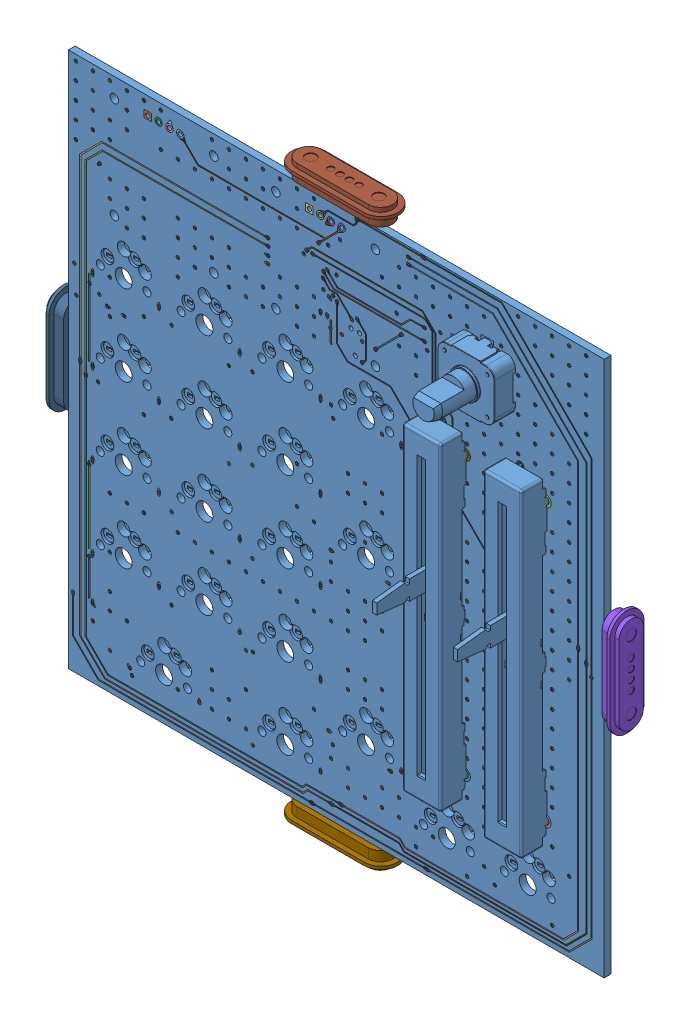
SolidWorks assembly Modulu1, configuration Default. Lengths in mm. (continued)
Components (placement in the parent): (continued)
- Numpad test 2.step-1: Numpad test 2.step [Default] at origin size (134.6 135 22.98) (continued)
  - Numpad test 21175.step-1: Numpad test 21175.step [Default] at origin size (0.81 0.81 0.01)
  - Numpad test 21176.step-1: Numpad test 21176.step [Default] at origin size (0.81 0.81 0.01)
  - Numpad test 21177.step-1: Numpad test 21177.step [Default] at origin size (0.81 0.81 0.01)
  - Numpad test 21178.step-1: Numpad test 21178.step [Default] at origin size (0.81 0.81 0.01)
  - Numpad test 21179.step-1: Numpad test 21179.step [Default] at origin size (0.81 0.81 0.01)
  - Numpad test 21180.step-1: Numpad test 21180.step [Default] at origin size (0.81 0.81 0.01)
  - Numpad test 21181.step-1: Numpad test 21181.step [Default] at origin size (0.81 0.81 0.01)
  - Numpad test 21182.step-1: Numpad test 21182.step [Default] at origin size (0.81 0.81 0.01)
  - Numpad test 21183.step-1: Numpad test 21183.step [Default] at origin size (0.81 0.81 0.01)
  - Numpad test 21184.step-1: Numpad test 21184.step [Default] at origin size (0.81 0.81 0.01)
  - Numpad test 21185.step-1: Numpad test 21185.step [Default] at origin size (0.81 0.81 0.01)
  - Numpad test 21186.step-1: Numpad test 21186.step [Default] at origin size (0.81 0.81 0.01)
  - Numpad test 21187.step-1: Numpad test 21187.step [Default] at origin size (0.81 0.81 0.01)
  - Numpad test 21188.step-1: Numpad test 21188.step [Default] at origin size (0.81 0.81 0.01)
  - Numpad test 21189.step-1: Numpad test 21189.step [Default] at origin size (0.81 0.81 0.01)
  - Numpad test 21190.step-1: Numpad test 21190.step [Default] at origin size (0.81 0.81 0.01)
  - Numpad test 21191.step-1: Numpad test 21191.step [Default] at origin size (0.81 0.81 0.01)
  - Numpad test 21192.step-1: Numpad test 21192.step [Default] at origin size (0.81 0.81 0.01)
  - Numpad test 21193.step-1: Numpad test 21193.step [Default] at origin size (0.81 0.81 0.01)
  - Numpad test 21194.step-1: Numpad test 21194.step [Default] at origin size (0.81 0.81 0.01)
  - Numpad test 21195.step-1: Numpad test 21195.step [Default] at origin size (0.81 0.81 0.01)
  - Numpad test 21196.step-1: Numpad test 21196.step [Default] at origin size (0.81 0.81 0.01)
  - Numpad test 21197.step-1: Numpad test 21197.step [Default] at origin size (0.81 0.81 0.01)
  - Numpad test 21198.step-1: Numpad test 21198.step [Default] at origin size (0.81 0.81 0.01)
  - Numpad test 21199.step-1: Numpad test 21199.step [Default] at origin size (0.81 0.81 0.01)
  - Numpad test 21200.step-1: Numpad test 21200.step [Default] at origin size (0.81 0.81 0.01)
  - Numpad test 21201.step-1: Numpad test 21201.step [Default] at origin size (0.81 0.81 0.01)
  - Numpad test 21202.step-1: Numpad test 21202.step [Default] at origin size (0.81 0.81 0.01)
  - Numpad test 21203.step-1: Numpad test 21203.step [Default] at origin size (0.81 0.81 0.01)
  - Numpad test 21204.step-1: Numpad test 21204.step [Default] at origin size (0.81 0.81 0.01)
  - Numpad test 21205.step-1: Numpad test 21205.step [Default] at origin size (0.81 0.81 0.01)
  - Numpad test 21206.step-1: Numpad test 21206.step [Default] at origin size (0.81 0.81 0.01)
  - Numpad test 21207.step-1: Numpad test 21207.step [Default] at origin size (0.81 0.81 0.01)
  - Numpad test 21208.step-1: Numpad test 21208.step [Default] at origin size (0.81 0.81 0.01)
  - Numpad test 21209.step-1: Numpad test 21209.step [Default] at origin size (0.81 0.81 0.01)
  - Numpad test 21210.step-1: Numpad test 21210.step [Default] at origin size (0.81 0.81 0.01)
  - Numpad test 21211.step-1: Numpad test 21211.step [Default] at origin size (0.81 0.81 0.01)
  - Numpad test 21212.step-1: Numpad test 21212.step [Default] at origin size (0.81 0.81 0.01)
  - Numpad test 21213.step-1: Numpad test 21213.step [Default] at origin size (0.81 0.81 0.01)
  - Numpad test 21214.step-1: Numpad test 21214.step [Default] at origin size (0.81 0.81 0.01)
  - Numpad test 21215.step-1: Numpad test 21215.step [Default] at origin size (0.81 0.81 0.01)
  - Numpad test 21216.step-1: Numpad test 21216.step [Default] at origin size (0.81 0.81 0.01)
  - Numpad test 21217.step-1: Numpad test 21217.step [Default] at origin size (0.81 0.81 0.01)
  - Numpad test 21218.step-1: Numpad test 21218.step [Default] at origin size (0.81 0.81 0.01)
  - Numpad test 21219.step-1: Numpad test 21219.step [Default] at origin size (0.81 0.81 0.01)
  - Numpad test 21220.step-1: Numpad test 21220.step [Default] at origin size (0.81 0.81 0.01)
  - Numpad test 21221.step-1: Numpad test 21221.step [Default] at origin size (0.81 0.81 0.01)
  - Numpad test 21222.step-1: Numpad test 21222.step [Default] at origin size (0.81 0.81 0.01)
  - Numpad test 21223.step-1: Numpad test 21223.step [Default] at origin size (0.81 0.81 0.01)
  - Numpad test 21224.step-1: Numpad test 21224.step [Default] at origin size (0.81 0.81 0.01)
  - Numpad test 21225.step-1: Numpad test 21225.step [Default] at origin size (0.81 0.81 0.01)
  - Numpad test 21226.step-1: Numpad test 21226.step [Default] at origin size (0.81 0.81 0.01)
  - Numpad test 21227.step-1: Numpad test 21227.step [Default] at origin size (0.81 0.81 0.01)
  - Numpad test 21228.step-1: Numpad test 21228.step [Default] at origin size (0.81 0.81 0.01)
  - Numpad test 21229.step-1: Numpad test 21229.step [Default] at origin size (0.81 0.81 0.01)
  - Numpad test 21230.step-1: Numpad test 21230.step [Default] at origin size (0.81 0.81 0.01)
  - Numpad test 21231.step-1: Numpad test 21231.step [Default] at origin size (0.81 0.81 0.01)
  - Numpad test 21232.step-1: Numpad test 21232.step [Default] at origin size (0.81 0.81 0.01)
  - Numpad test 21233.step-1: Numpad test 21233.step [Default] at origin size (0.81 0.81 0.01)
  - Numpad test 21234.step-1: Numpad test 21234.step [Default] at origin size (0.81 0.81 0.01)
  - Numpad test 21235.step-1: Numpad test 21235.step [Default] at origin size (0.81 0.81 0.01)
  - Numpad test 21236.step-1: Numpad test 21236.step [Default] at origin size (0.81 0.81 0.01)
  - Numpad test 21237.step-1: Numpad test 21237.step [Default] at origin size (0.81 0.81 0.01)
  - Numpad test 21238.step-1: Numpad test 21238.step [Default] at origin size (0.81 0.81 0.01)
  - Numpad test 21239.step-1: Numpad test 21239.step [Default] at origin size (0.81 0.81 0.01)
  - Numpad test 21240.step-1: Numpad test 21240.step [Default] at origin size (0.81 0.81 0.01)
  - Numpad test 21241.step-1: Numpad test 21241.step [Default] at origin size (0.81 0.81 0.01)
  - Numpad test 21242.step-1: Numpad test 21242.step [Default] at origin size (0.81 0.81 0.01)
  - Numpad test 21243.step-1: Numpad test 21243.step [Default] at origin size (0.81 0.81 0.01)
  - Numpad test 21244.step-1: Numpad test 21244.step [Default] at origin size (0.81 0.81 0.01)
  - Numpad test 21245.step-1: Numpad test 21245.step [Default] at origin size (0.81 0.81 0.01)
  - Numpad test 21246.step-1: Numpad test 21246.step [Default] at origin size (0.81 0.81 0.01)
  - Numpad test 21247.step-1: Numpad test 21247.step [Default] at origin size (0.81 0.81 0.01)
  - Numpad test 21248.step-1: Numpad test 21248.step [Default] at origin size (0.81 0.81 0.01)
  - Numpad test 21249.step-1: Numpad test 21249.step [Default] at origin size (0.81 0.81 0.01)
  - Numpad test 21250.step-1: Numpad test 21250.step [Default] at origin size (0.81 0.81 0.01)
  - Numpad test 21251.step-1: Numpad test 21251.step [Default] at origin size (0.81 0.81 0.01)
  - Numpad test 21252.step-1: Numpad test 21252.step [Default] at origin size (0.81 0.81 0.01)
  - Numpad test 21253.step-1: Numpad test 21253.step [Default] at origin size (0.81 0.81 0.01)
  - Numpad test 21254.step-1: Numpad test 21254.step [Default] at origin size (0.81 0.81 0.01)
  - Numpad test 21255.step-1: Numpad test 21255.step [Default] at origin size (0.81 0.81 0.01)
  - Numpad test 21256.step-1: Numpad test 21256.step [Default] at origin size (0.81 0.81 0.01)
  - Numpad test 21257.step-1: Numpad test 21257.step [Default] at origin size (0.81 0.81 0.01)
  - Numpad test 21258.step-1: Numpad test 21258.step [Default] at origin size (0.81 0.81 0.01)
  - Numpad test 21259.step-1: Numpad test 21259.step [Default] at origin size (0.81 0.81 0.01)
  - Numpad test 21260.step-1: Numpad test 21260.step [Default] at origin size (0.81 0.81 0.01)
  - Numpad test 21261.step-1: Numpad test 21261.step [Default] at origin size (0.81 0.81 0.01)
  - Numpad test 21262.step-1: Numpad test 21262.step [Default] at origin size (0.81 0.81 0.01)
  - Numpad test 21263.step-1: Numpad test 21263.step [Default] at origin size (0.81 0.81 0.01)
  - Numpad test 21264.step-1: Numpad test 21264.step [Default] at origin size (0.81 0.81 0.01)
  - Numpad test 21265.step-1: Numpad test 21265.step [Default] at origin size (0.81 0.81 0.01)
  - Numpad test 21266.step-1: Numpad test 21266.step [Default] at origin size (0.81 0.81 0.01)
  - Numpad test 21267.step-1: Numpad test 21267.step [Default] at origin size (0.81 0.81 0.01)
  - Numpad test 21268.step-1: Numpad test 21268.step [Default] at origin size (0.81 0.81 0.01)
  - Numpad test 21269.step-1: Numpad test 21269.step [Default] at origin size (0.81 0.81 0.01)
  - Numpad test 21270.step-1: Numpad test 21270.step [Default] at origin size (0.81 0.81 0.01)
  - Numpad test 21271.step-1: Numpad test 21271.step [Default] at origin size (0.81 0.81 0.01)
  - Numpad test 21272.step-1: Numpad test 21272.step [Default] at origin size (0.81 0.81 0.01)
  - Numpad test 21273.step-1: Numpad test 21273.step [Default] at origin size (0.81 0.81 0.01)
  - Numpad test 21274.step-1: Numpad test 21274.step [Default] at origin size (0.81 0.81 0.01)
  - Numpad test 21275.step-1: Numpad test 21275.step [Default] at origin size (0.81 0.81 0.01)
  - Numpad test 21276.step-1: Numpad test 21276.step [Default] at origin size (0.81 0.81 0.01)
  - Numpad test 21277.step-1: Numpad test 21277.step [Default] at origin size (0.81 0.81 0.01)
  - Numpad test 21278.step-1: Numpad test 21278.step [Default] at origin size (0.81 0.81 0.01)
  - Numpad test 21279.step-1: Numpad test 21279.step [Default] at origin size (0.81 0.81 0.01)
  - Numpad test 21280.step-1: Numpad test 21280.step [Default] at origin size (0.81 0.81 0.01)
  - Numpad test 21281.step-1: Numpad test 21281.step [Default] at origin size (0.81 0.81 0.01)
  - Numpad test 21282.step-1: Numpad test 21282.step [Default] at origin size (0.81 0.81 0.01)
  - Numpad test 21283.step-1: Numpad test 21283.step [Default] at origin size (0.81 0.81 0.01)
  - Numpad test 21284.step-1: Numpad test 21284.step [Default] at origin size (0.81 0.81 0.01)
  - Numpad test 21285.step-1: Numpad test 21285.step [Default] at origin size (0.81 0.81 0.01)
  - Numpad test 21286.step-1: Numpad test 21286.step [Default] at origin size (0.81 0.81 0.01)
  - Numpad test 21287.step-1: Numpad test 21287.step [Default] at origin size (0.81 0.81 0.01)
  - Numpad test 21288.step-1: Numpad test 21288.step [Default] at origin size (0.81 0.81 0.01)
  - Numpad test 21289.step-1: Numpad test 21289.step [Default] at origin size (0.81 0.81 0.01)
  - Numpad test 21290.step-1: Numpad test 21290.step [Default] at origin size (0.81 0.81 0.01)
  - Numpad test 21291.step-1: Numpad test 21291.step [Default] at origin size (0.81 0.81 0.01)
  - Numpad test 21292.step-1: Numpad test 21292.step [Default] at origin size (0.81 0.81 0.01)
  - Numpad test 21293.step-1: Numpad test 21293.step [Default] at origin size (0.81 0.81 0.01)
  - Numpad test 21294.step-1: Numpad test 21294.step [Default] at origin size (0.81 0.81 0.01)
  - Numpad test 21295.step-1: Numpad test 21295.step [Default] at origin size (0.81 0.81 0.01)
  - Numpad test 21296.step-1: Numpad test 21296.step [Default] at origin size (0.81 0.81 0.01)
  - Numpad test 21297.step-1: Numpad test 21297.step [Default] at origin size (0.81 0.81 0.01)
  - Numpad test 21298.step-1: Numpad test 21298.step [Default] at origin size (0.81 0.81 0.01)
  - Numpad test 21299.step-1: Numpad test 21299.step [Default] at origin size (0.81 0.81 0.01)
  - Numpad test 21300.step-1: Numpad test 21300.step [Default] at origin size (0.81 0.81 0.01)
  - Numpad test 21301.step-1: Numpad test 21301.step [Default] at origin size (0.81 0.81 0.01)
  - Numpad test 21302.step-1: Numpad test 21302.step [Default] at origin size (0.81 0.81 0.01)
  - Numpad test 21303.step-1: Numpad test 21303.step [Default] at origin size (0.81 0.81 0.01)
  - Numpad test 21304.step-1: Numpad test 21304.step [Default] at origin size (0.81 0.81 0.01)
  - Numpad test 21305.step-1: Numpad test 21305.step [Default] at origin size (0.81 0.81 0.01)
  - Numpad test 21306.step-1: Numpad test 21306.step [Default] at origin size (0.81 0.81 0.01)
  - Numpad test 21307.step-1: Numpad test 21307.step [Default] at origin size (0.81 0.81 0.01)
  - Numpad test 21308.step-1: Numpad test 21308.step [Default] at origin size (0.81 0.81 0.01)
  - Numpad test 21309.step-1: Numpad test 21309.step [Default] at origin size (0.81 0.81 0.01)
  - Numpad test 21310.step-1: Numpad test 21310.step [Default] at origin size (0.81 0.81 0.01)
  - Numpad test 21311.step-1: Numpad test 21311.step [Default] at origin size (0.81 0.81 0.01)
  - Numpad test 21312.step-1: Numpad test 21312.step [Default] at origin size (0.81 0.81 0.01)
  - Numpad test 21313.step-1: Numpad test 21313.step [Default] at origin size (0.81 0.81 0.01)
  - Numpad test 21314.step-1: Numpad test 21314.step [Default] at origin size (0.81 0.81 0.01)
  - Numpad test 21315.step-1: Numpad test 21315.step [Default] at origin size (0.81 0.81 0.01)
  - Numpad test 21316.step-1: Numpad test 21316.step [Default] at origin size (0.81 0.81 0.01)
  - Numpad test 21317.step-1: Numpad test 21317.step [Default] at origin size (0.81 0.81 0.01)
  - Numpad test 21318.step-1: Numpad test 21318.step [Default] at origin size (0.81 0.81 0.01)
  - Numpad test 21319.step-1: Numpad test 21319.step [Default] at origin size (0.81 0.81 0.01)
  - Numpad test 21320.step-1: Numpad test 21320.step [Default] at origin size (0.81 0.81 0.01)
  - Numpad test 21321.step-1: Numpad test 21321.step [Default] at origin size (0.81 0.81 0.01)
  - Numpad test 21322.step-1: Numpad test 21322.step [Default] at origin size (0.81 0.81 0.01)
  - Numpad test 21323.step-1: Numpad test 21323.step [Default] at origin size (0.81 0.81 0.01)
  - Numpad test 21324.step-1: Numpad test 21324.step [Default] at origin size (0.81 0.81 0.01)
  - Numpad test 21325.step-1: Numpad test 21325.step [Default] at origin size (0.81 0.81 0.01)
  - Numpad test 21326.step-1: Numpad test 21326.step [Default] at origin size (0.81 0.81 0.01)
  - Numpad test 21327.step-1: Numpad test 21327.step [Default] at origin size (0.81 0.81 0.01)
  - Numpad test 21328.step-1: Numpad test 21328.step [Default] at origin size (0.81 0.81 0.01)
  - Numpad test 21329.step-1: Numpad test 21329.step [Default] at origin size (0.81 0.81 0.01)
  - Numpad test 21330.step-1: Numpad test 21330.step [Default] at origin size (0.81 0.81 0.01)
  - Numpad test 21331.step-1: Numpad test 21331.step [Default] at origin size (0.81 0.81 0.01)
  - Numpad test 21332.step-1: Numpad test 21332.step [Default] at origin size (0.81 0.81 0.01)
  - Numpad test 21333.step-1: Numpad test 21333.step [Default] at origin size (0.81 0.81 0.01)
  - Numpad test 21334.step-1: Numpad test 21334.step [Default] at origin size (0.81 0.81 0.01)
  - Numpad test 21335.step-1: Numpad test 21335.step [Default] at origin size (0.81 0.81 0.01)
  - Numpad test 21336.step-1: Numpad test 21336.step [Default] at origin size (0.81 0.81 0.01)
  - Numpad test 21337.step-1: Numpad test 21337.step [Default] at origin size (0.81 0.81 0.01)
  - Numpad test 21338.step-1: Numpad test 21338.step [Default] at origin size (0.81 0.81 0.01)
  - Numpad test 21339.step-1: Numpad test 21339.step [Default] at origin size (0.81 0.81 0.01)
  - Numpad test 21340.step-1: Numpad test 21340.step [Default] at origin size (0.81 0.81 0.01)
  - Numpad test 21341.step-1: Numpad test 21341.step [Default] at origin size (0.81 0.81 0.01)
  - Numpad test 21342.step-1: Numpad test 21342.step [Default] at origin size (0.81 0.81 0.01)
  - Numpad test 21343.step-1: Numpad test 21343.step [Default] at origin size (0.81 0.81 0.01)
  - Numpad test 21344.step-1: Numpad test 21344.step [Default] at origin size (0.81 0.81 0.01)
  - Numpad test 21345.step-1: Numpad test 21345.step [Default] at origin size (0.81 0.81 0.01)
  - Numpad test 21346.step-1: Numpad test 21346.step [Default] at origin size (0.81 0.81 0.01)
  - Numpad test 21347.step-1: Numpad test 21347.step [Default] at origin size (0.81 0.81 0.01)
  - Numpad test 21348.step-1: Numpad test 21348.step [Default] at origin size (0.81 0.81 0.01)
  - Numpad test 21349.step-1: Numpad test 21349.step [Default] at origin size (0.81 0.81 0.01)
  - Numpad test 21350.step-1: Numpad test 21350.step [Default] at origin size (0.81 0.81 0.01)
  - Numpad test 21351.step-1: Numpad test 21351.step [Default] at origin size (0.81 0.81 0.01)
  - Numpad test 21352.step-1: Numpad test 21352.step [Default] at origin size (0.81 0.81 0.01)
  - Numpad test 21353.step-1: Numpad test 21353.step [Default] at origin size (0.81 0.81 0.01)
  - Numpad test 21354.step-1: Numpad test 21354.step [Default] at origin size (0.81 0.81 0.01)
  - Numpad test 21355.step-1: Numpad test 21355.step [Default] at origin size (0.81 0.81 0.01)
  - Numpad test 21356.step-1: Numpad test 21356.step [Default] at origin size (0.81 0.81 0.01)
  - Numpad test 21357.step-1: Numpad test 21357.step [Default] at origin size (0.81 0.81 0.01)
  - Numpad test 21358.step-1: Numpad test 21358.step [Default] at origin size (0.81 0.81 0.01)
  - Numpad test 21359.step-1: Numpad test 21359.step [Default] at origin size (0.81 0.81 0.01)
  - Numpad test 21360.step-1: Numpad test 21360.step [Default] at origin size (0.81 0.81 0.01)
  - Numpad test 21361.step-1: Numpad test 21361.step [Default] at origin size (0.81 0.81 0.01)
  - Numpad test 21362.step-1: Numpad test 21362.step [Default] at origin size (0.81 0.81 0.01)
  - Numpad test 21363.step-1: Numpad test 21363.step [Default] at origin size (0.81 0.81 0.01)
  - Numpad test 21364.step-1: Numpad test 21364.step [Default] at origin size (0.81 0.81 0.01)
  - Numpad test 21365.step-1: Numpad test 21365.step [Default] at origin size (0.81 0.81 0.01)
  - Numpad test 21366.step-1: Numpad test 21366.step [Default] at origin size (0.81 0.81 0.01)
  - Numpad test 21367.step-1: Numpad test 21367.step [Default] at origin size (0.81 0.81 0.01)
  - Numpad test 21368.step-1: Numpad test 21368.step [Default] at origin size (0.81 0.81 0.01)
  - Numpad test 21369.step-1: Numpad test 21369.step [Default] at origin size (0.81 0.81 0.01)
  - Numpad test 21370.step-1: Numpad test 21370.step [Default] at origin size (0.81 0.81 0.01)
  - Numpad test 21371.step-1: Numpad test 21371.step [Default] at origin size (0.81 0.81 0.01)
  - Numpad test 21372.step-1: Numpad test 21372.step [Default] at origin size (0.81 0.81 0.01)
  - Numpad test 21373.step-1: Numpad test 21373.step [Default] at origin size (0.81 0.81 0.01)
  - Numpad test 21374.step-1: Numpad test 21374.step [Default] at origin size (0.81 0.81 0.01)
  - Numpad test 21375.step-1: Numpad test 21375.step [Default] at origin size (0.81 0.81 0.01)
  - Numpad test 21376.step-1: Numpad test 21376.step [Default] at origin size (0.81 0.81 0.01)
  - Numpad test 21377.step-1: Numpad test 21377.step [Default] at origin size (0.81 0.81 0.01)
  - Numpad test 21378.step-1: Numpad test 21378.step [Default] at origin size (0.81 0.81 0.01)
  - Numpad test 21379.step-1: Numpad test 21379.step [Default] at origin size (0.81 0.81 0.01)
  - Numpad test 21380.step-1: Numpad test 21380.step [Default] at origin size (0.81 0.81 0.01)
  - Numpad test 21381.step-1: Numpad test 21381.step [Default] at origin size (0.81 0.81 0.01)
  - Numpad test 21382.step-1: Numpad test 21382.step [Default] at origin size (0.81 0.81 0.01)
  - Numpad test 21383.step-1: Numpad test 21383.step [Default] at origin size (0.81 0.81 0.01)
  - Numpad test 21384.step-1: Numpad test 21384.step [Default] at origin size (0.81 0.81 0.01)
  - Numpad test 21385.step-1: Numpad test 21385.step [Default] at origin size (0.81 0.81 0.01)
  - Numpad test 21386.step-1: Numpad test 21386.step [Default] at origin size (0.81 0.81 0.01)
  - Numpad test 21387.step-1: Numpad test 21387.step [Default] at origin size (0.81 0.81 0.01)
  - Numpad test 21388.step-1: Numpad test 21388.step [Default] at origin size (0.81 0.81 0.01)
  - Numpad test 21389.step-1: Numpad test 21389.step [Default] at origin size (0.81 0.81 0.01)
  - Numpad test 21390.step-1: Numpad test 21390.step [Default] at origin size (0.81 0.81 0.01)
  - Numpad test 21391.step-1: Numpad test 21391.step [Default] at origin size (0.81 0.81 0.01)
  - Numpad test 21392.step-1: Numpad test 21392.step [Default] at origin size (0.81 0.81 0.01)
  - Numpad test 21393.step-1: Numpad test 21393.step [Default] at origin size (0.81 0.81 0.01)
  - Numpad test 21394.step-1: Numpad test 21394.step [Default] at origin size (0.81 0.81 0.01)
  - Numpad test 21395.step-1: Numpad test 21395.step [Default] at origin size (0.81 0.81 0.01)
  - Numpad test 21396.step-1: Numpad test 21396.step [Default] at origin size (0.81 0.81 0.01)
  - Numpad test 21397.step-1: Numpad test 21397.step [Default] at origin size (0.81 0.81 0.01)
  - Numpad test 21398.step-1: Numpad test 21398.step [Default] at origin size (0.81 0.81 0.01)
  - Numpad test 21399.step-1: Numpad test 21399.step [Default] at origin size (0.81 0.81 0.01)
  - Numpad test 21400.step-1: Numpad test 21400.step [Default] at origin size (0.81 0.81 0.01)
  - Numpad test 21401.step-1: Numpad test 21401.step [Default] at origin size (0.81 0.81 0.01)
  - Numpad test 21402.step-1: Numpad test 21402.step [Default] at origin size (0.81 0.81 0.01)
  - Numpad test 21403.step-1: Numpad test 21403.step [Default] at origin size (0.81 0.81 0.01)
  - Numpad test 21404.step-1: Numpad test 21404.step [Default] at origin size (0.81 0.81 0.01)
  - Numpad test 21405.step-1: Numpad test 21405.step [Default] at origin size (0.81 0.81 0.01)
  - Numpad test 21406.step-1: Numpad test 21406.step [Default] at origin size (0.81 0.81 0.01)
  - Numpad test 21407.step-1: Numpad test 21407.step [Default] at origin size (0.81 0.81 0.01)
  - Numpad test 21408.step-1: Numpad test 21408.step [Default] at origin size (0.81 0.81 0.01)
  - Numpad test 21409.step-1: Numpad test 21409.step [Default] at origin size (0.81 0.81 0.01)
  - Numpad test 21410.step-1: Numpad test 21410.step [Default] at origin size (0.81 0.81 0.01)
  - Numpad test 21411.step-1: Numpad test 21411.step [Default] at origin size (0.81 0.81 0.01)
  - Numpad test 21412.step-1: Numpad test 21412.step [Default] at origin size (0.81 0.81 0.01)
  - Numpad test 21413.step-1: Numpad test 21413.step [Default] at origin size (0.81 0.81 0.01)
  - Numpad test 21414.step-1: Numpad test 21414.step [Default] at origin size (0.81 0.81 0.01)
  - Numpad test 21415.step-1: Numpad test 21415.step [Default] at origin size (0.81 0.81 0.01)
  - Numpad test 21416.step-1: Numpad test 21416.step [Default] at origin size (0.81 0.81 0.01)
  - Numpad test 21417.step-1: Numpad test 21417.step [Default] at origin size (0.81 0.81 0.01)
  - Numpad test 21418.step-1: Numpad test 21418.step [Default] at origin size (0.81 0.81 0.01)
  - Numpad test 21419.step-1: Numpad test 21419.step [Default] at origin size (0.81 0.81 0.01)
  - Numpad test 21420.step-1: Numpad test 21420.step [Default] at origin size (0.81 0.81 0.01)
  - Numpad test 21421.step-1: Numpad test 21421.step [Default] at origin size (0.81 0.81 0.01)
  - Numpad test 21422.step-1: Numpad test 21422.step [Default] at origin size (0.81 0.81 0.01)
  - Numpad test 21423.step-1: Numpad test 21423.step [Default] at origin size (1.01 0.51 0.01)
  - Numpad test 21424.step-1: Numpad test 21424.step [Default] at origin size (1.01 0.51 0.01)
  - Numpad test 21425.step-1: Numpad test 21425.step [Default] at origin size (1.01 0.51 0.01)
  - Numpad test 21426.step-1: Numpad test 21426.step [Default] at origin size (1.01 0.51 0.01)
  - Numpad test 21427.step-1: Numpad test 21427.step [Default] at origin size (1.01 0.51 0.01)
  - Numpad test 21428.step-1: Numpad test 21428.step [Default] at origin size (1.01 0.51 0.01)
  - Numpad test 21429.step-1: Numpad test 21429.step [Default] at origin size (0.8 0.8 0.01)
  - Numpad test 21430.step-1: Numpad test 21430.step [Default] at origin size (0.8 0.8 0.01)
  - Numpad test 21431.step-1: Numpad test 21431.step [Default] at origin size (0.8 0.8 0.01)
  - Numpad test 21432.step-1: Numpad test 21432.step [Default] at origin size (0.8 0.8 0.01)
  - Numpad test 21433.step-1: Numpad test 21433.step [Default] at origin size (0.8 0.8 0.01)
  - Numpad test 21434.step-1: Numpad test 21434.step [Default] at origin size (0.8 0.8 0.01)
  - Numpad test 21435.step-1: Numpad test 21435.step [Default] at origin size (0.26 0.68 0.01)
  - Numpad test 21436.step-1: Numpad test 21436.step [Default] at origin size (0.26 3.04 0.01)
  - Numpad test 21437.step-1: Numpad test 21437.step [Default] at origin size (2.27 1.78 0.01)
  - Numpad test 21438.step-1: Numpad test 21438.step [Default] at origin size (0.19 0.19 0.01)
  - Numpad test 21439.step-1: Numpad test 21439.step [Default] at origin size (0.26 0.12 0.01)
  - Numpad test 21440.step-1: Numpad test 21440.step [Default] at origin size (0.26 0.21 0.01)
  - Numpad test 21441.step-1: Numpad test 21441.step [Default] at origin size (36.27 52.47 0.01)
  - Numpad test 21442.step-1: Numpad test 21442.step [Default] at origin size (2.18 0.96 0.01)
  - Numpad test 21443.step-1: Numpad test 21443.step [Default] at origin size (0.98 1.02 0.01)
  - Numpad test 21444.step-1: Numpad test 21444.step [Default] at origin size (0.26 0.12 0.01)
  - Numpad test 21445.step-1: Numpad test 21445.step [Default] at origin size (0.26 0.21 0.01)
  - Numpad test 21446.step-1: Numpad test 21446.step [Default] at origin size (0.19 0.26 0.01)
  - Numpad test 21447.step-1: Numpad test 21447.step [Default] at origin size (0.66 0.66 0.01)
  - Numpad test 21448.step-1: Numpad test 21448.step [Default] at origin size (0.42 0.26 0.01)
  - Numpad test 21449.step-1: Numpad test 21449.step [Default] at origin size (2.06 0.26 0.01)
  - Numpad test 21450.step-1: Numpad test 21450.step [Default] at origin size (68.41 3.24 0.01)
  - Numpad test 21451.step-1: Numpad test 21451.step [Default] at origin size (0.68 0.26 0.01)
  - Numpad test 21452.step-1: Numpad test 21452.step [Default] at origin size (0.26 0.88 0.01)
  - Numpad test 21453.step-1: Numpad test 21453.step [Default] at origin size (0.26 0.22 0.01)
  - Numpad test 21454.step-1: Numpad test 21454.step [Default] at origin size (53.45 13.32 0.01)
  - Numpad test 21455.step-1: Numpad test 21455.step [Default] at origin size (0.26 1.25 0.01)
  - Numpad test 21456.step-1: Numpad test 21456.step [Default] at origin size (1.08 3.3 0.01)
  - Numpad test 21457.step-1: Numpad test 21457.step [Default] at origin size (0.2 0.19 0.01)
  - Numpad test 21458.step-1: Numpad test 21458.step [Default] at origin size (0.13 0.58 0.01)
  - Numpad test 21459.step-1: Numpad test 21459.step [Default] at origin size (2.66 6.31 0.01)
  - Numpad test 21460.step-1: Numpad test 21460.step [Default] at origin size (0.13 0.58 0.01)
  - Numpad test 21461.step-1: Numpad test 21461.step [Default] at origin size (0.33 1.29 0.01)
  - Numpad test 21462.step-1: Numpad test 21462.step [Default] at origin size (0.07 0.13 0.01)
  - Numpad test 21463.step-1: Numpad test 21463.step [Default] at origin size (0.28 2.58 0.01)
  - Numpad test 21464.step-1: Numpad test 21464.step [Default] at origin size (0.44 3.01 0.01)
  - Numpad test 21465.step-1: Numpad test 21465.step [Default] at origin size (0.09 0.14 0.01)
  - Numpad test 21466.step-1: Numpad test 21466.step [Default] at origin size (0.13 0.58 0.01)
  - Numpad test 21467.step-1: Numpad test 21467.step [Default] at origin size (0.26 0.21 0.01)
  - Numpad test 21468.step-1: Numpad test 21468.step [Default] at origin size (0.66 0.66 0.01)
  - Numpad test 21469.step-1: Numpad test 21469.step [Default] at origin size (0.13 0.58 0.01)
  - Numpad test 21470.step-1: Numpad test 21470.step [Default] at origin size (0.46 0.33 0.01)
  - Numpad test 21471.step-1: Numpad test 21471.step [Default] at origin size (0.09 0.14 0.01)
  - Numpad test 21472.step-1: Numpad test 21472.step [Default] at origin size (0.26 0.68 0.01)
  - Numpad test 21473.step-1: Numpad test 21473.step [Default] at origin size (19.96 33.21 0.01)
  - Numpad test 21474.step-1: Numpad test 21474.step [Default] at origin size (1.4 0.26 0.01)
  - Numpad test 21475.step-1: Numpad test 21475.step [Default] at origin size (0.36 0.26 0.01)
  - Numpad test 21476.step-1: Numpad test 21476.step [Default] at origin size (0.26 0.68 0.01)
  - Numpad test 21477.step-1: Numpad test 21477.step [Default] at origin size (17.62 16.56 0.01)
  - Numpad test 21478.step-1: Numpad test 21478.step [Default] at origin size (0.26 0.68 0.01)
  - Numpad test 21479.step-1: Numpad test 21479.step [Default] at origin size (2.03 1.05 0.01)
  - Numpad test 21480.step-1: Numpad test 21480.step [Default] at origin size (0.19 0.18 0.01)
  - Numpad test 21481.step-1: Numpad test 21481.step [Default] at origin size (0.33 0.26 0.01)
  - Numpad test 21482.step-1: Numpad test 21482.step [Default] at origin size (0.97 1.21 0.01)
  - Numpad test 21483.step-1: Numpad test 21483.step [Default] at origin size (0.19 0.25 0.01)
  - Numpad test 21484.step-1: Numpad test 21484.step [Default] at origin size (0.26 0.67 0.01)
  - Numpad test 21485.step-1: Numpad test 21485.step [Default] at origin size (1.52 0.92 0.01)
  - Numpad test 21486.step-1: Numpad test 21486.step [Default] at origin size (0.25 0.23 0.01)
  - Numpad test 21487.step-1: Numpad test 21487.step [Default] at origin size (0.53 0.23 0.01)
  - Numpad test 21488.step-1: Numpad test 21488.step [Default] at origin size (0.13 0.26 0.01)
  - Numpad test 21489.step-1: Numpad test 21489.step [Default] at origin size (1.04 0.96 0.01)
  - Numpad test 21490.step-1: Numpad test 21490.step [Default] at origin size (0.21 0.21 0.01)
  - Numpad test 21491.step-1: Numpad test 21491.step [Default] at origin size (0.26 0.09 0.01)
  - Numpad test 21492.step-1: Numpad test 21492.step [Default] at origin size (0.26 0.86 0.01)
  - Numpad test 21493.step-1: Numpad test 21493.step [Default] at origin size (0.26 0.21 0.01)
  - Numpad test 21494.step-1: Numpad test 21494.step [Default] at origin size (0.66 0.66 0.01)
  - Numpad test 21495.step-1: Numpad test 21495.step [Default] at origin size (16.82 2.72 0.01)
  - Numpad test 21496.step-1: Numpad test 21496.step [Default] at origin size (0.91 0.31 0.01)
  - Numpad test 21497.step-1: Numpad test 21497.step [Default] at origin size (0.23 0.26 0.01)
  - Numpad test 21498.step-1: Numpad test 21498.step [Default] at origin size (14.62 1.84 0.01)
  - Numpad test 21499.step-1: Numpad test 21499.step [Default] at origin size (0.66 0.66 0.01)
  - Numpad test 21500.step-1: Numpad test 21500.step [Default] at origin size (0.91 0.31 0.01)
  - Numpad test 21501.step-1: Numpad test 21501.step [Default] at origin size (0.23 0.26 0.01)
  - Numpad test 21502.step-1: Numpad test 21502.step [Default] at origin size (0.36 0.26 0.01)
  - Numpad test 21503.step-1: Numpad test 21503.step [Default] at origin size (1.4 0.26 0.01)
  - Numpad test 21504.step-1: Numpad test 21504.step [Default] at origin size (10.64 1.76 0.01)
  - Numpad test 21505.step-1: Numpad test 21505.step [Default] at origin size (1.4 0.26 0.01)
  - Numpad test 21506.step-1: Numpad test 21506.step [Default] at origin size (0.36 0.26 0.01)
  - Numpad test 21507.step-1: Numpad test 21507.step [Default] at origin size (0.36 0.26 0.01)
  - Numpad test 21508.step-1: Numpad test 21508.step [Default] at origin size (1.4 0.26 0.01)
  - Numpad test 21509.step-1: Numpad test 21509.step [Default] at origin size (10.64 1.76 0.01)
  - Numpad test 21510.step-1: Numpad test 21510.step [Default] at origin size (1.4 0.26 0.01)
  - Numpad test 21511.step-1: Numpad test 21511.step [Default] at origin size (0.36 0.26 0.01)
  - Numpad test 21512.step-1: Numpad test 21512.step [Default] at origin size (0.26 0.42 0.01)
  - Numpad test 21513.step-1: Numpad test 21513.step [Default] at origin size (0.26 1.11 0.01)
  - Numpad test 21514.step-1: Numpad test 21514.step [Default] at origin size (2.19 5.84 0.01)
  - Numpad test 21515.step-1: Numpad test 21515.step [Default] at origin size (0.26 1.25 0.01)
  - Numpad test 21516.step-1: Numpad test 21516.step [Default] at origin size (0.61 0.38 0.01)
  - Numpad test 21517.step-1: Numpad test 21517.step [Default] at origin size (0.32 0.42 0.01)
  - Numpad test 21518.step-1: Numpad test 21518.step [Default] at origin size (5.2 0.32 0.01)
  - Numpad test 21519.step-1: Numpad test 21519.step [Default] at origin size (2.47 0.26 0.01)
  - Numpad test 21520.step-1: Numpad test 21520.step [Default] at origin size (0.39 0.26 0.01)
  - Numpad test 21521.step-1: Numpad test 21521.step [Default] at origin size (0.8 0.81 0.01)
  - Numpad test 21522.step-1: Numpad test 21522.step [Default] at origin size (0.26 0.26 0.01)
  - Numpad test 21523.step-1: Numpad test 21523.step [Default] at origin size (2.99 7.29 0.02)
  - Numpad test 21524.step-1: Numpad test 21524.step [Default] at origin size (0.85 0.26 0.01)
  - Numpad test 21525.step-1: Numpad test 21525.step [Default] at origin size (0.16 0.26 0.01)
  - Numpad test 21526.step-1: Numpad test 21526.step [Default] at origin size (1.18 0.26 0.01)
  - Numpad test 21527.step-1: Numpad test 21527.step [Default] at origin size (0.43 0.26 0.01)
  - Numpad test 21528.step-1: Numpad test 21528.step [Default] at origin size (0.26 0.42 0.01)
  - Numpad test 21529.step-1: Numpad test 21529.step [Default] at origin size (0.26 1.11 0.01)
  - Numpad test 21530.step-1: Numpad test 21530.step [Default] at origin size (1.79 3.42 0.01)
  - Numpad test 21531.step-1: Numpad test 21531.step [Default] at origin size (1.56 1.56 0.01)
  - Numpad test 21532.step-1: Numpad test 21532.step [Default] at origin size (0.29 0.29 0.01)
  - Numpad test 21533.step-1: Numpad test 21533.step [Default] at origin size (0.68 0.26 0.01)
  - Numpad test 21534.step-1: Numpad test 21534.step [Default] at origin size (2.81 0.26 0.01)
  - Numpad test 21535.step-1: Numpad test 21535.step [Default] at origin size (1.69 0.26 0.01)
  - Numpad test 21536.step-1: Numpad test 21536.step [Default] at origin size (0.42 0.26 0.01)
  - Numpad test 21537.step-1: Numpad test 21537.step [Default] at origin size (0.16 0.26 0.01)
  - Numpad test 21538.step-1: Numpad test 21538.step [Default] at origin size (0.85 0.26 0.01)
  - Numpad test 21539.step-1: Numpad test 21539.step [Default] at origin size (0.85 3.89 0.01)
  - Numpad test 21540.step-1: Numpad test 21540.step [Default] at origin size (0.26 1.11 0.01)
  - Numpad test 21541.step-1: Numpad test 21541.step [Default] at origin size (0.26 0.42 0.01)
  - Numpad test 21542.step-1: Numpad test 21542.step [Default] at origin size (0.16 0.26 0.01)
  - Numpad test 21543.step-1: Numpad test 21543.step [Default] at origin size (0.85 0.26 0.01)
  - Numpad test 21544.step-1: Numpad test 21544.step [Default] at origin size (2.8 2.01 0.01)
  - Numpad test 21545.step-1: Numpad test 21545.step [Default] at origin size (0.66 0.66 0.01)
  - Numpad test 21546.step-1: Numpad test 21546.step [Default] at origin size (1.85 0.27 0.01)
  - Numpad test 21547.step-1: Numpad test 21547.step [Default] at origin size (0.24 0.29 0.01)
  - Numpad test 21548.step-1: Numpad test 21548.step [Default] at origin size (1.95 1.28 0.01)
  - Numpad test 21549.step-1: Numpad test 21549.step [Default] at origin size (0.21 0.26 0.01)
  - Numpad test 21550.step-1: Numpad test 21550.step [Default] at origin size (0.09 0.06 0.01)
  - Numpad test 21551.step-1: Numpad test 21551.step [Default] at origin size (0.21 0.26 0.01)
  - Numpad test 21552.step-1: Numpad test 21552.step [Default] at origin size (1.95 1.08 0.01)
  - Numpad test 21553.step-1: Numpad test 21553.step [Default] at origin size (0.28 0.07 0.01)
  - Numpad test 21554.step-1: Numpad test 21554.step [Default] at origin size (1.85 0.26 0.01)
  - Numpad test 21555.step-1: Numpad test 21555.step [Default] at origin size (0.21 0.26 0.01)
  - Numpad test 21556.step-1: Numpad test 21556.step [Default] at origin size (0.21 0.26 0.01)
  - Numpad test 21557.step-1: Numpad test 21557.step [Default] at origin size (0.86 0.26 0.01)
  - Numpad test 21558.step-1: Numpad test 21558.step [Default] at origin size (0.86 0.26 0.01)
  - Numpad test 21559.step-1: Numpad test 21559.step [Default] at origin size (2.6 0.26 0.01)
  - Numpad test 21560.step-1: Numpad test 21560.step [Default] at origin size (0.58 0.13 0.01)
  - Numpad test 21561.step-1: Numpad test 21561.step [Default] at origin size (0.58 0.13 0.01)
  - Numpad test 21562.step-1: Numpad test 21562.step [Default] at origin size (1.48 2.08 0.01)
  - Numpad test 21563.step-1: Numpad test 21563.step [Default] at origin size (1.56 1.42 0.01)
  - Numpad test 21564.step-1: Numpad test 21564.step [Default] at origin size (0.26 0.42 0.01)
  - Numpad test 21565.step-1: Numpad test 21565.step [Default] at origin size (0.26 1.11 0.01)
  - Numpad test 21566.step-1: Numpad test 21566.step [Default] at origin size (1.81 1.79 0.01)
  - Numpad test 21567.step-1: Numpad test 21567.step [Default] at origin size (0.68 0.26 0.01)
  - Numpad test 21568.step-1: Numpad test 21568.step [Default] at origin size (0.26 0.34 0.01)
  - Numpad test 21569.step-1: Numpad test 21569.step [Default] at origin size (2.08 0.59 0.01)
  - Numpad test 21570.step-1: Numpad test 21570.step [Default] at origin size (0.42 0.17 0.01)
  - Numpad test 21571.step-1: Numpad test 21571.step [Default] at origin size (0.15 0.08 0.01)
  - Numpad test 21572.step-1: Numpad test 21572.step [Default] at origin size (0.3 1.94 0.01)
  - Numpad test 21573.step-1: Numpad test 21573.step [Default] at origin size (0.61 0.85 0.01)
  - Numpad test 21574.step-1: Numpad test 21574.step [Default] at origin size (0.05 0.29 0.01)
  - Numpad test 21575.step-1: Numpad test 21575.step [Default] at origin size (0.26 0.24 0.01)
  - Numpad test 21576.step-1: Numpad test 21576.step [Default] at origin size (0.56 2.79 0.01)
  - Numpad test 21577.step-1: Numpad test 21577.step [Default] at origin size (1.98 0.57 0.01)
  - Numpad test 21578.step-1: Numpad test 21578.step [Default] at origin size (0.3 0.15 0.01)
  - Numpad test 21579.step-1: Numpad test 21579.step [Default] at origin size (0.43 0.27 0.01)
  - Numpad test 21580.step-1: Numpad test 21580.step [Default] at origin size (0.2 0.26 0.01)
  - Numpad test 21581.step-1: Numpad test 21581.step [Default] at origin size (0.26 0.42 0.01)
  - Numpad test 21582.step-1: Numpad test 21582.step [Default] at origin size (0.26 1.69 0.01)
  - Numpad test 21583.step-1: Numpad test 21583.step [Default] at origin size (0.26 1.11 0.01)
  - Numpad test 21584.step-1: Numpad test 21584.step [Default] at origin size (0.26 0.68 0.01)
  - Numpad test 21585.step-1: Numpad test 21585.step [Default] at origin size (0.68 0.26 0.01)
  - Numpad test 21586.step-1: Numpad test 21586.step [Default] at origin size (0.91 0.26 0.01)
  - Numpad test 21587.step-1: Numpad test 21587.step [Default] at origin size (1.69 0.26 0.01)
  - Numpad test 21588.step-1: Numpad test 21588.step [Default] at origin size (0.42 0.26 0.01)
  - Numpad test 21589.step-1: Numpad test 21589.step [Default] at origin size (0.24 0.24 0.01)
  - Numpad test 21590.step-1: Numpad test 21590.step [Default] at origin size (0.74 0.75 0.01)
  - Numpad test 21591.step-1: Numpad test 21591.step [Default] at origin size (0.34 2.16 0.01)
  - Numpad test 21592.step-1: Numpad test 21592.step [Default] at origin size (0.66 0.66 0.01)
  - Numpad test 21593.step-1: Numpad test 21593.step [Default] at origin size (0.26 0.42 0.01)
  - Numpad test 21594.step-1: Numpad test 21594.step [Default] at origin size (0.26 1.69 0.01)
  - Numpad test 21595.step-1: Numpad test 21595.step [Default] at origin size (0.26 0.11 0.01)
  - Numpad test 21596.step-1: Numpad test 21596.step [Default] at origin size (0.26 0.68 0.01)
  - Numpad test 21597.step-1: Numpad test 21597.step [Default] at origin size (1.18 0.26 0.01)
  - Numpad test 21598.step-1: Numpad test 21598.step [Default] at origin size (0.43 0.26 0.01)
  - Numpad test 21599.step-1: Numpad test 21599.step [Default] at origin size (0.39 1.51 0.02)
  - Numpad test 21600.step-1: Numpad test 21600.step [Default] at origin size (0.51 0.65 0.01)
  - Numpad test 21601.step-1: Numpad test 21601.step [Default] at origin size (0.05 0.21 0.02)
  - Numpad test 21602.step-1: Numpad test 21602.step [Default] at origin size (0.76 0.76 0.01)
  - Numpad test 21603.step-1: Numpad test 21603.step [Default] at origin size (0.86 0.26 0.01)
  - Numpad test 21604.step-1: Numpad test 21604.step [Default] at origin size (0.22 0.26 0.01)
  - Numpad test 21605.step-1: Numpad test 21605.step [Default] at origin size (0.68 0.26 0.01)
  - Numpad test 21606.step-1: Numpad test 21606.step [Default] at origin size (0.29 0.21 0.01)
  - Numpad test 21607.step-1: Numpad test 21607.step [Default] at origin size (0.27 2.5 0.01)
  - Numpad test 21608.step-1: Numpad test 21608.step [Default] at origin size (0.26 0.26 0.01)
  - Numpad test 21609.step-1: Numpad test 21609.step [Default] at origin size (0.21 0.19 0.01)
  - Numpad test 21610.step-1: Numpad test 21610.step [Default] at origin size (0.27 2.39 0.01)
  - Numpad test 21611.step-1: Numpad test 21611.step [Default] at origin size (0.26 0.26 0.01)
  - Numpad test 21612.step-1: Numpad test 21612.step [Default] at origin size (0.21 0.19 0.01)
  - Numpad test 21613.step-1: Numpad test 21613.step [Default] at origin size (0.27 2.39 0.01)
  - Numpad test 21614.step-1: Numpad test 21614.step [Default] at origin size (0.26 0.26 0.01)
  - Numpad test 21615.step-1: Numpad test 21615.step [Default] at origin size (0.66 0.66 0.01)
  - Numpad test 21616.step-1: Numpad test 21616.step [Default] at origin size (1.39 0.64 0.01)
  - Numpad test 21617.step-1: Numpad test 21617.step [Default] at origin size (0.64 0.54 0.02)
  - Numpad test 21618.step-1: Numpad test 21618.step [Default] at origin size (0.47 0.47 0.02)
  - Numpad test 21619.step-1: Numpad test 21619.step [Default] at origin size (0.35 1.14 0.01)
  - Numpad test 21620.step-1: Numpad test 21620.step [Default] at origin size (0.06 0.08 0.01)
  - Numpad test 21621.step-1: Numpad test 21621.step [Default] at origin size (0.26 0.54 0.01)
  - Numpad test 21622.step-1: Numpad test 21622.step [Default] at origin size (0.32 0.64 0.02)
  - Numpad test 21623.step-1: Numpad test 21623.step [Default] at origin size (0.27 1.21 0.02)
  - Numpad test 21624.step-1: Numpad test 21624.step [Default] at origin size (0.26 0.44 0.01)
  - Numpad test 21625.step-1: Numpad test 21625.step [Default] at origin size (0.61 1.54 0.01)
  - Numpad test 21626.step-1: Numpad test 21626.step [Default] at origin size (0.64 0.68 0.01)
  - Numpad test 21627.step-1: Numpad test 21627.step [Default] at origin size (0.25 0.25 0.01)
  - Numpad test 21628.step-1: Numpad test 21628.step [Default] at origin size (0.66 0.61 0.01)
  - Numpad test 21629.step-1: Numpad test 21629.step [Default] at origin size (0.39 0.24 0.01)
  - Numpad test 21630.step-1: Numpad test 21630.step [Default] at origin size (0.22 0.26 0.01)
  - Numpad test 21631.step-1: Numpad test 21631.step [Default] at origin size (1.37 0.26 0.01)
  - Numpad test 21632.step-1: Numpad test 21632.step [Default] at origin size (0.26 0.25 0.01)
  - Numpad test 21633.step-1: Numpad test 21633.step [Default] at origin size (0.35 0.59 0.01)
  - Numpad test 21634.step-1: Numpad test 21634.step [Default] at origin size (0.39 0.5 0.01)
  - Numpad test 21635.step-1: Numpad test 21635.step [Default] at origin size (0.68 0.29 0.01)
  - Numpad test 21636.step-1: Numpad test 21636.step [Default] at origin size (0.68 0.26 0.01)
  - Numpad test 21637.step-1: Numpad test 21637.step [Default] at origin size (0.42 0.47 0.01)
  - Numpad test 21638.step-1: Numpad test 21638.step [Default] at origin size (0.28 0.62 0.01)
  - Numpad test 21639.step-1: Numpad test 21639.step [Default] at origin size (0.26 0.23 0.01)
  - Numpad test 21640.step-1: Numpad test 21640.step [Default] at origin size (0.26 1.19 0.01)
  - Numpad test 21641.step-1: Numpad test 21641.step [Default] at origin size (0.26 0.2 0.01)
  - Numpad test 21642.step-1: Numpad test 21642.step [Default] at origin size (0.26 1.09 0.01)
  - Numpad test 21643.step-1: Numpad test 21643.step [Default] at origin size (0.26 0.2 0.01)
  - Numpad test 21644.step-1: Numpad test 21644.step [Default] at origin size (1.05 0.26 0.01)
  - Numpad test 21645.step-1: Numpad test 21645.step [Default] at origin size (0.1 0.06 0.01)
  - Numpad test 21646.step-1: Numpad test 21646.step [Default] at origin size (1 0.26 0.01)
  - Numpad test 21647.step-1: Numpad test 21647.step [Default] at origin size (75.17 7.02 0.02)
  - Numpad test 21648.step-1: Numpad test 21648.step [Default] at origin size (64.71 3.45 0.02)
  - Numpad test 21649.step-1: Numpad test 21649.step [Default] at origin size (9.63 17.63 0.02)
  - Numpad test 21650.step-1: Numpad test 21650.step [Default] at origin size (15.65 1.66 0.02)
  - Numpad test 21651.step-1: Numpad test 21651.step [Default] at origin size (2.78 6.17 0)
  - Numpad test 21652.step-1: Numpad test 21652.step [Default] at origin size (5.93 1.76 0.02)
  - Numpad test 21653.step-1: Numpad test 21653.step [Default] at origin size (5.93 1.76 0.02)
  - Numpad test 21654.step-1: Numpad test 21654.step [Default] at origin size (5.93 1.76 0.02)
  - Numpad test 21655.step-1: Numpad test 21655.step [Default] at origin size (5.88 1.73 0.02)
  - Numpad test 21656.step-1: Numpad test 21656.step [Default] at origin size (5.88 1.73 0.02)
  - Numpad test 21657.step-1: Numpad test 21657.step [Default] at origin size (5.75 1.66 0.02)
  - Numpad test 21658.step-1: Numpad test 21658.step [Default] at origin size (5.75 1.66 0.02)
  - Numpad test 21659.step-1: Numpad test 21659.step [Default] at origin size (5.65 1.56 0.01)
  - Numpad test 21660.step-1: Numpad test 21660.step [Default] at origin size (5.65 1.56 0.01)
  - Numpad test 21661.step-1: Numpad test 21661.step [Default] at origin size (3.02 4.89 0.02)
  - Numpad test 21662.step-1: Numpad test 21662.step [Default] at origin size (4.41 3.19 0.02)
  - Numpad test 21663.step-1: Numpad test 21663.step [Default] at origin size (4.47 3.1 0.02)
  - Numpad test 21664.step-1: Numpad test 21664.step [Default] at origin size (4.47 3.1 0.02)
  - Numpad test 21665.step-1: Numpad test 21665.step [Default] at origin size (4.18 3.43 0.01)
  - Numpad test 21666.step-1: Numpad test 21666.step [Default] at origin size (4.21 3.35 0.01)
  - Numpad test 21667.step-1: Numpad test 21667.step [Default] at origin size (4.21 3.35 0.01)
  - Numpad test 21668.step-1: Numpad test 21668.step [Default] at origin size (4.21 3.35 0.01)
  - Numpad test 21669.step-1: Numpad test 21669.step [Default] at origin size (4.21 3.35 0.01)
  - Numpad test 21670.step-1: Numpad test 21670.step [Default] at origin size (4.21 3.35 0.01)
  - Numpad test 21671.step-1: Numpad test 21671.step [Default] at origin size (4.21 3.35 0.01)
  - Numpad test 21672.step-1: Numpad test 21672.step [Default] at origin size (4.21 3.35 0.01)
  - Numpad test 21673.step-1: Numpad test 21673.step [Default] at origin size (4.21 3.35 0.01)
  - Numpad test 21674.step-1: Numpad test 21674.step [Default] at origin size (4.21 3.35 0.01)
  - Numpad test 21675.step-1: Numpad test 21675.step [Default] at origin size (4.42 3.05 0.01)
  - Numpad test 21676.step-1: Numpad test 21676.step [Default] at origin size (0.76 0.31 0.01)
  - Numpad test 21677.step-1: Numpad test 21677.step [Default] at origin size (3.31 1.18 0)
  - Numpad test 21678.step-1: Numpad test 21678.step [Default] at origin size (1.69 1.48 0)
  - Numpad test 21679.step-1: Numpad test 21679.step [Default] at origin size (2.05 0.86 0)
  - Numpad test 21680.step-1: Numpad test 21680.step [Default] at origin size (4.85 1.66 0.02)
  - Numpad test 21681.step-1: Numpad test 21681.step [Default] at origin size (3.22 3.95 0.01)
  - Numpad test 21682.step-1: Numpad test 21682.step [Default] at origin size (2.16 4.48 0)
  - Numpad test 21683.step-1: Numpad test 21683.step [Default] at origin size (3.45 3.45 0.02)
  - Numpad test 21684.step-1: Numpad test 21684.step [Default] at origin size (3.15 3.66 0.01)
  - Numpad test 21685.step-1: Numpad test 21685.step [Default] at origin size (4.19 2.27 0.01)
  - Numpad test 21686.step-1: Numpad test 21686.step [Default] at origin size (3.37 2.4 0.01)
  - Numpad test 21687.step-1: Numpad test 21687.step [Default] at origin size (3.37 2.4 0.01)
  - Numpad test 21688.step-1: Numpad test 21688.step [Default] at origin size (3.39 2.34 0.01)
  - Numpad test 21689.step-1: Numpad test 21689.step [Default] at origin size (3.39 2.28 0.02)
  - Numpad test 21690.step-1: Numpad test 21690.step [Default] at origin size (3.39 2.28 0.02)
  - Numpad test 21691.step-1: Numpad test 21691.step [Default] at origin size (3.22 2.48 0.01)
  - Numpad test 21692.step-1: Numpad test 21692.step [Default] at origin size (3.12 2.47 0.01)
  - Numpad test 21693.step-1: Numpad test 21693.step [Default] at origin size (0.18 0.82 0.01)
  - Numpad test 21694.step-1: Numpad test 21694.step [Default] at origin size (0.18 0.82 0.01)
  - Numpad test 21695.step-1: Numpad test 21695.step [Default] at origin size (0.36 1.54 0.01)
  - Numpad test 21696.step-1: Numpad test 21696.step [Default] at origin size (0.83 1.74 0.01)
  - Numpad test 21697.step-1: Numpad test 21697.step [Default] at origin size (0.71 0.34 0.01)
  - Numpad test 21698.step-1: Numpad test 21698.step [Default] at origin size (2.62 2.33 0.01)
  - Numpad test 21699.step-1: Numpad test 21699.step [Default] at origin size (1.69 1.79 0)
  - Numpad test 21700.step-1: Numpad test 21700.step [Default] at origin size (1.59 0.99 0)
  - Numpad test 21701.step-1: Numpad test 21701.step [Default] at origin size (0.83 0.37 0.01)
  - Numpad test 21702.step-1: Numpad test 21702.step [Default] at origin size (1.66 0.83 0.01)
  - Numpad test 21703.step-1: Numpad test 21703.step [Default] at origin size (0.36 0.9 0.01)
  - Numpad test 21704.step-1: Numpad test 21704.step [Default] at origin size (1.54 0.36 0.01)
  - Numpad test 21705.step-1: Numpad test 21705.step [Default] at origin size (0.38 0.64 0.01)
  - Numpad test 21706.step-1: Numpad test 21706.step [Default] at origin size (0.43 0.71 0.01)
  - Numpad test 21707.step-1: Numpad test 21707.step [Default] at origin size (2.59 2.19 0.02)
  - Numpad test 21708.step-1: Numpad test 21708.step [Default] at origin size (2.59 2.13 0.02)
  - Numpad test 21709.step-1: Numpad test 21709.step [Default] at origin size (2.05 2.51 0.01)
  - Numpad test 21710.step-1: Numpad test 21710.step [Default] at origin size (2.05 2.5 0.01)
  - Numpad test 21711.step-1: Numpad test 21711.step [Default] at origin size (0.91 2.28 0.01)
  - Numpad test 21712.step-1: Numpad test 21712.step [Default] at origin size (0.91 2.26 0.01)
  - Numpad test 21713.step-1: Numpad test 21713.step [Default] at origin size (2.21 2.32 0.01)
  - Numpad test 21714.step-1: Numpad test 21714.step [Default] at origin size (2.27 2.27 0.01)
  - Numpad test 21715.step-1: Numpad test 21715.step [Default] at origin size (2.27 2.27 0.01)
  - Numpad test 21716.step-1: Numpad test 21716.step [Default] at origin size (2.27 2.27 0.01)
  - Numpad test 21717.step-1: Numpad test 21717.step [Default] at origin size (2.27 2.27 0.01)
  - Numpad test 21718.step-1: Numpad test 21718.step [Default] at origin size (2.27 2.27 0.01)
  - Numpad test 21719.step-1: Numpad test 21719.step [Default] at origin size (2.93 1.25 0.02)
  - Numpad test 21720.step-1: Numpad test 21720.step [Default] at origin size (2.93 1.25 0.02)
  - Numpad test 21721.step-1: Numpad test 21721.step [Default] at origin size (2.93 1.25 0.02)
  - Numpad test 21722.step-1: Numpad test 21722.step [Default] at origin size (2.05 2.41 0.01)
  - Numpad test 21723.step-1: Numpad test 21723.step [Default] at origin size (2.05 2.41 0.01)
  - Numpad test 21724.step-1: Numpad test 21724.step [Default] at origin size (2.05 2.41 0.02)
  - Numpad test 21725.step-1: Numpad test 21725.step [Default] at origin size (2.05 2.41 0.02)
  - Numpad test 21726.step-1: Numpad test 21726.step [Default] at origin size (2.05 2.41 0.02)
  - Numpad test 21727.step-1: Numpad test 21727.step [Default] at origin size (2.05 2.41 0.01)
  - Numpad test 21728.step-1: Numpad test 21728.step [Default] at origin size (2.05 2.41 0.01)
  - Numpad test 21729.step-1: Numpad test 21729.step [Default] at origin size (2.05 2.4 0.01)
  - Numpad test 21730.step-1: Numpad test 21730.step [Default] at origin size (2.05 2.4 0.01)
  - Numpad test 21731.step-1: Numpad test 21731.step [Default] at origin size (2.05 2.4 0.01)
  - Numpad test 21732.step-1: Numpad test 21732.step [Default] at origin size (2.05 2.4 0.01)
  - Numpad test 21733.step-1: Numpad test 21733.step [Default] at origin size (0.98 2.26 0.02)
  - Numpad test 21734.step-1: Numpad test 21734.step [Default] at origin size (0.92 2.1 0.01)
  - Numpad test 21735.step-1: Numpad test 21735.step [Default] at origin size (0.98 2.26 0.02)
  - Numpad test 21736.step-1: Numpad test 21736.step [Default] at origin size (0.92 2.1 0.01)
  - Numpad test 21737.step-1: Numpad test 21737.step [Default] at origin size (0.18 1.41 0.01)
  - Numpad test 21738.step-1: Numpad test 21738.step [Default] at origin size (0.48 1.53 0.01)
  - Numpad test 21739.step-1: Numpad test 21739.step [Default] at origin size (0.18 0.82 0.01)
  - Numpad test 21740.step-1: Numpad test 21740.step [Default] at origin size (0.18 0.82 0.01)
  - Numpad test 21741.step-1: Numpad test 21741.step [Default] at origin size (2.42 0.91 0.01)
  - Numpad test 21742.step-1: Numpad test 21742.step [Default] at origin size (2.19 0.79 0.01)
  - Numpad test 21743.step-1: Numpad test 21743.step [Default] at origin size (2.35 2.05 0.01)
  - Numpad test 21744.step-1: Numpad test 21744.step [Default] at origin size (0.5 0.67 0)
  - Numpad test 21745.step-1: Numpad test 21745.step [Default] at origin size (1.86 0.3 0)
  - Numpad test 21746.step-1: Numpad test 21746.step [Default] at origin size (2.02 2.18 0.01)
  - Numpad test 21747.step-1: Numpad test 21747.step [Default] at origin size (2.17 1.98 0.01)
  - Numpad test 21748.step-1: Numpad test 21748.step [Default] at origin size (2.56 1.33 0.01)
  - Numpad test 21749.step-1: Numpad test 21749.step [Default] at origin size (1.94 2.12 0.01)
  - Numpad test 21750.step-1: Numpad test 21750.step [Default] at origin size (1.86 0.93 0)
  - Numpad test 21751.step-1: Numpad test 21751.step [Default] at origin size (1.9 0.93 0)
